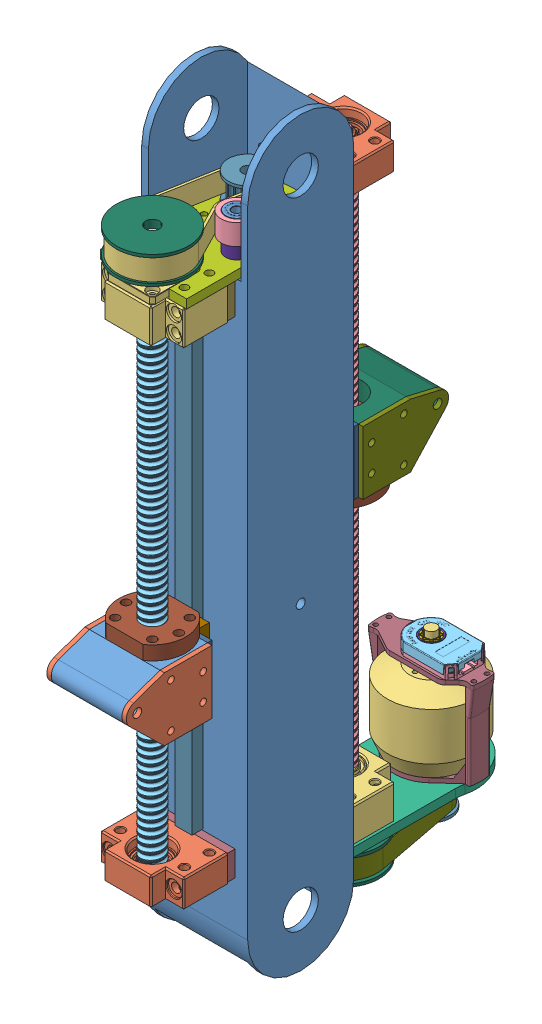
SolidWorks assembly Shoulder, configuration Default. Lengths in mm.
Overall size (98.94 610.39 280.38).
79 component instances, 40 part files, 66 mates.
Components (placement in the parent):
- Box^Shoulder-1: Box^Shoulder [Default] at origin size (76.2 533.4 76.2) (virtual)
- BF12-1: BF12 [Default] at (0 614.1315 -46.7041) x (1 0 0) z (0 1 0) size (60 43 20)
- BK12-1: BK12 [Default] at (0 212.1315 -46.7041) x (-1 0 0) z (0 -1 0) size (60 46.94 35.34)
- SFU1605-450-1: SFU1605-450 [1605-400] at (0 171.1315 -71.7041) x (1 0 0) z (0 -1 0) size (16.52 16.22 450)
- BK12-2: BK12 [Default] at (0 582.269 40.2909) x (-1 0 0) z (0 1 0) size (60 46.94 35.34)
- BF12-2: BF12 [Default] at (0 230.269 40.2909) x (-1 0 0) z (0 1 0) size (60 43 20)
- SFU1605-400-3: SFU1605-400 [1605-400] at (0 623.269 65.2909) x (-1 0 0) z (0 1 0) size (16.52 16.22 400)
- J3Plate^Shoulder-1: J3Plate^Shoulder [Default] at origin size (65 6.35 120.35) (virtual)
- J2Plate^Shoulder-1: J2Plate^Shoulder [Default] at origin size (66.67 6.35 116.57) (virtual)
- J3MGN12R-1: J3MGN12R [Default] at origin size (12 379.5 8)
- J3MGN12C-1: J3MGN12C [Default] at (0 433.1293 -49.3066) x (1 0 0) z (0 1 0) size (27 10 45.5)
- CarriagePlate^Shoulder-1: CarriagePlate^Shoulder [Default] at (0 67.1524 -3.2066) size (50.8 45.5 3.17) (virtual)
- nut-1: nut [Default] at (0 410.3793 -71.7041) x (-1 0 0) z (0 -1 0) size (48 40 42)
- BKSpacer^Shoulder-1: BKSpacer^Shoulder [Default] at origin size (58 23 5.4) (virtual)
- BKSpacer^Shoulder-2: BKSpacer^Shoulder [Default] at (0 370.1375 81.5975) size (58 23 5.4) (virtual)
- BFSpacer^Shoulder-1: BFSpacer^Shoulder [Default] at origin size (58 18 5.4) (virtual)
- BFSpacer^Shoulder-2: BFSpacer^Shoulder [Default] at (0 -383.8625 81.5975) size (58 18 5.4) (virtual)
- J2MGN12R^Shoulder-1: J2MGN12R^Shoulder [Default] at origin size (12 329.5 8) (virtual)
- J3Adapter^Shoulder-2: J3Adapter^Shoulder [Default] at (0 76.5186 -3.2066) size (57.15 45.79 61.61) (virtual)
  - Body^J3Adapter_Shoulder-1: Body^J3Adapter_Shoulder [Default] at (38.1 26.927 0) x (0 0 -1) z (1 0 0) size (61.61 45.5 50.8) (virtual)
  - SidePlate^J3Adapter_Shoulder-1: SidePlate^J3Adapter_Shoulder [Default] at origin size (3.18 45.5 61.61) (virtual)
  - SidePlate^J3Adapter_Shoulder-2: SidePlate^J3Adapter_Shoulder [Default] at (53.975 0 0) size (3.18 45.5 61.61) (virtual)
  - 94459A340_BRASS HEAT-SET INSERT FOR PLASTIC-1: 94459A340_BRASS HEAT-SET INSERT FOR PLASTIC [94459A340] at (-18.415 340.7357 -83.735) x (0 -1 0) z (0 0 -1) size (7.22 6.55 7.22)
  - 94459A220_BRASS HEAT-SET INSERT FOR PLASTIC-1: 94459A220_BRASS HEAT-SET INSERT FOR PLASTIC [94459A220] at (13.435 346.5607 -81.9325) x (-0.837169 0 -0.546944) z (-0.546944 0 0.837169) size (8.76 13.2 8.76)
- J3MGN12C-2: J3MGN12C [Default] at (0 351.2303 42.8934) x (-1 0 0) z (0 1 0) size (27 10 45.5)
- nut-2: nut [Default] at (0 373.9803 65.2909) x (1 0 0) z (0 1 0) size (48 40 42)
- J2Adapter^Shoulder-1: J2Adapter^Shoulder [Default] at (0 707.841 -3.2066) x (1 0 0) z (0 0 -1) size (57.15 457.2 153.99) (virtual)
  - Body^J2Adapter_Shoulder-1: Body^J2Adapter_Shoulder [Default] at (38.1 26.927 0) x (0 0 -1) z (1 0 0) size (61.61 45.5 50.8) (virtual)
  - SidePlate^J2Adapter_Shoulder-1: SidePlate^J2Adapter_Shoulder [Default] at origin size (3.18 45.5 61.61) (virtual)
  - SidePlate^J2Adapter_Shoulder-2: SidePlate^J2Adapter_Shoulder [Default] at (53.975 0 0) size (3.18 45.5 61.61) (virtual)
  - 94459A340_BRASS HEAT-SET INSERT FOR PLASTIC-1: 94459A340_BRASS HEAT-SET INSERT FOR PLASTIC [94459A340] at (-18.415 340.7357 -83.735) x (0 -1 0) z (0 0 -1) size (7.22 6.55 7.22)
  - 94459A220_BRASS HEAT-SET INSERT FOR PLASTIC-1: 94459A220_BRASS HEAT-SET INSERT FOR PLASTIC [94459A220] at (13.435 346.5607 -81.9325) x (-0.837169 0 -0.546944) z (-0.546944 0 0.837169) size (8.76 13.2 8.76)
- CarriagePlate^Shoulder-2: CarriagePlate^Shoulder [Default] at (0 -14.7465 -3.2066) x (-1 0 0) z (0 0 -1) size (50.8 45.5 3.17) (virtual)
- 192kvMotorEncoded-1: 192kvMotorEncoded [Default] at (0 202.8065 -135.2041) x (0 0 -1) z (1 0 0) size (63 104.52 76.93)
  - BetterKEDA-1: BetterKEDA [Default] at origin size (63 104.52 63)
  - CUI_DEVICES_AMT102-0048-N2000-S-1: CUI_DEVICES_AMT102-0048-N2000-S [Default] at (0 65.12 0) x (1 0 0) z (0 1 0) size (36.33 46.21 9.2)
    - CUI_DEVICES_AMT102-0048-N2000-S.step-1: CUI_DEVICES_AMT102-0048-N2000-S.step [Default] at origin size (36.33 46.21 9.2)
      - AMT-102-Base-REV-K.step-1: AMT-102-Base-REV-K.step [Default] x (-1 0 0) z (0 0 -1) size (28.78 43.39 9.06)
      - AMT-102-Top-Cover-REV-H.step-1: AMT-102-Top-Cover-REV-H.step [Default] at (0 0 5.23) x (-1 0 0) z (0 0 -1) size (28.6 43.26 6.55)
      - AMT-Sleeve-REV-D_ 2 mm.step-1: AMT-Sleeve-REV-D_ 2 mm.step [Default] at (0 0 -2.42) x (0.999996 0.002864 0) z (0 0 1) size (10.79 10.79 7.8)
      - AMT-Hub-Top-REV-D1.step-1: AMT-Hub-Top-REV-D1.step [Default] at (0 0 2.13) x (0.999996 0.002864 0) z (0 0 1) size (14 14 5.67)
      - AMT-Hub-Bottom-REV-B.step-1: AMT-Hub-Bottom-REV-B.step [Default] at (0 0 2.43) x (0.999998 -0.001942 0) z (0 0 1) size (17.3 17.3 3.2)
      - AMT10X-Shaft-Adaptor-REV-E.step-1: AMT10X-Shaft-Adaptor-REV-E.step [Default] at (0 0 0.03) x (0.999996 0.002864 0) z (0 0 1) size (11.8 11.8 7.8)
      - Receiver-board.step-1: Receiver-board.step [Default] at (72.2834 -20.351 3.03) x (-1 0 0) z (0 0 -1) size (26.5 26.62 0.41)
      - Rotor-board-REV F.step-1: Rotor-board-REV F.step [Default] at (0 0 2.13) x (0.807874 -0.589355 0) z (0 0 1) size (26 26 0.3)
      - Transmitter-board AMT10_AMT-102.step-1: Transmitter-board AMT10_AMT-102.step [Default] at (19.1596 -17.1102 1.22) x (-1 0 0) z (0 0 -1) size (26.63 38.43 4.41)
  - Body^192kvMotorEncoded-1: Body^192kvMotorEncoded [Default] at origin size (53 64.53 76.93) (virtual)
- 192kvMotorEncoded-2: 192kvMotorEncoded [Default] at (0 591.594 -3.2066) x (-0.707107 0 -0.707107) z (-0.707107 0 0.707107) size (63 104.52 76.93)
  - BetterKEDA-1: BetterKEDA [Default] at origin size (63 104.52 63)
  - CUI_DEVICES_AMT102-0048-N2000-S-1: CUI_DEVICES_AMT102-0048-N2000-S [Default] at (0 65.12 0) x (1 0 0) z (0 1 0) size (36.33 46.21 9.2)
    - CUI_DEVICES_AMT102-0048-N2000-S.step-1: CUI_DEVICES_AMT102-0048-N2000-S.step [Default] at origin size (36.33 46.21 9.2)
      - AMT-102-Base-REV-K.step-1: AMT-102-Base-REV-K.step [Default] x (-1 0 0) z (0 0 -1) size (28.78 43.39 9.06)
      - AMT-102-Top-Cover-REV-H.step-1: AMT-102-Top-Cover-REV-H.step [Default] at (0 0 5.23) x (-1 0 0) z (0 0 -1) size (28.6 43.26 6.55)
      - AMT-Sleeve-REV-D_ 2 mm.step-1: AMT-Sleeve-REV-D_ 2 mm.step [Default] at (0 0 -2.42) x (0.999996 0.002864 0) z (0 0 1) size (10.79 10.79 7.8)
      - AMT-Hub-Top-REV-D1.step-1: AMT-Hub-Top-REV-D1.step [Default] at (0 0 2.13) x (0.999996 0.002864 0) z (0 0 1) size (14 14 5.67)
      - AMT-Hub-Bottom-REV-B.step-1: AMT-Hub-Bottom-REV-B.step [Default] at (0 0 2.43) x (0.999998 -0.001942 0) z (0 0 1) size (17.3 17.3 3.2)
      - AMT10X-Shaft-Adaptor-REV-E.step-1: AMT10X-Shaft-Adaptor-REV-E.step [Default] at (0 0 0.03) x (0.999996 0.002864 0) z (0 0 1) size (11.8 11.8 7.8)
      - Receiver-board.step-1: Receiver-board.step [Default] at (72.2834 -20.351 3.03) x (-1 0 0) z (0 0 -1) size (26.5 26.62 0.41)
      - Rotor-board-REV F.step-1: Rotor-board-REV F.step [Default] at (0 0 2.13) x (0.807874 -0.589355 0) z (0 0 1) size (26 26 0.3)
      - Transmitter-board AMT10_AMT-102.step-1: Transmitter-board AMT10_AMT-102.step [Default] at (19.1596 -17.1102 1.22) x (-1 0 0) z (0 0 -1) size (26.63 38.43 4.41)
  - Body^192kvMotorEncoded-1: Body^192kvMotorEncoded [Default] at origin size (53 64.53 76.93) (virtual)
- 15Tpulley-3: 15Tpulley [Default] at (0 175.8815 -135.2041) size (28 28 28)
- 15Tpulley-4: 15Tpulley [Default] at (0 618.519 -3.2066) x (-1 0 0) z (0 0 1) size (28 28 28)
- 30Tpulley-3: 30Tpulley [Default] at (0 618.519 65.2909) size (52 20 52)
- 30Tpulley-4: 30Tpulley [Default] at (0 175.8815 -71.7041) size (52 20 52)
- J3Belt^Shoulder-1: J3Belt^Shoulder [Default] at origin size (49.49 15 101.05) (virtual)
- TensionPillarJ3-1: TensionPillarJ3 [Default] at (-42.5291 257.8915 3.8215) size (22.22 25.73 22.23)
  - 92510A774_ALUM UNTHRD SPACER-1-1: 92510A774_ALUM UNTHRD SPACER-1 [92510A774] at (20.3041 -69.3725 -110.4505) x (1 0 0) z (0 1 0) size (15.88 15.88 9.53)
  - 98019A228_MIL SPEC. 300 SERIES SS FLAT WASHER-1: 98019A228_MIL SPEC. 300 SERIES SS FLAT WASHER [98019A228] at (20.3041 -74.8462 -110.4505) x (0.972939 0 -0.231063) z (0.231063 0 0.972939) size (9.53 0.71 9.53)
  - 60355K701_BALL BEARING-1: 60355K701_BALL BEARING [60355K701] at (20.3041 -77.3354 -110.4505) x (1 0 0) z (0 1 0) size (15.88 15.88 4.98)
  - Roller^TensionPillarJ3-1: Roller^TensionPillarJ3 [Default] at (-2.0675 -17.1652 2.6827) size (22.23 15 22.23) (virtual)
  - 60355K701_BALL BEARING-2: 60355K701_BALL BEARING [60355K701] at (20.3041 -87.8548 -110.4505) x (1 0 0) z (0 1 0) size (15.88 15.88 4.98)
- J2Belt^Shoulder-1: J2Belt^Shoulder [Default] at origin size (49.49 15 106.05) (virtual)
- TensionPillarJ2-1: TensionPillarJ2 [Default] at (-24.3623 536.509 127.3519) x (-0.837169 0 -0.546944) z (-0.546944 0 0.837169) size (22.22 25.73 22.23)
  - 92510A774_ALUM UNTHRD SPACER-1-1: 92510A774_ALUM UNTHRD SPACER-1 [92510A774] at (20.3041 -69.3725 -110.4505) x (1 0 0) z (0 1 0) size (15.88 15.88 9.53)
  - 98019A228_MIL SPEC. 300 SERIES SS FLAT WASHER-1: 98019A228_MIL SPEC. 300 SERIES SS FLAT WASHER [98019A228] at (20.3041 -74.8462 -110.4505) x (0.972939 0 -0.231063) z (0.231063 0 0.972939) size (9.53 0.71 9.53)
  - 60355K701_BALL BEARING-1: 60355K701_BALL BEARING [60355K701] at (20.3041 -77.3354 -110.4505) x (1 0 0) z (0 1 0) size (15.88 15.88 4.98)
  - Roller^TensionPillarJ2-1: Roller^TensionPillarJ2 [Default] at (-2.0675 -17.1652 2.6827) size (22.23 15 22.23) (virtual)
  - 60355K701_BALL BEARING-2: 60355K701_BALL BEARING [60355K701] at (20.3041 -87.8548 -110.4505) x (1 0 0) z (0 1 0) size (15.88 15.88 4.98)
Mates (geometry in assembly coordinates):
- Parallel1: parallel anti-aligned: plane of Box^Shoulder-1 through (-33.3375 186.9315 -41.3066) normal (0 0 -1); plane of BF12-1 through (29 605.1315 -46.7041) normal (0 0 1)
- Width1: width anti-aligned: plane of BF12-1 through (30 605.1315 -78.2041) normal (1 0 0); plane of Box^Shoulder-1 through (-30 605.1315 -47.7041) normal (-1 0 0); plane of BF12-1 through (38.1 644.1315 -3.2066) normal (1 0 0); plane of Box^Shoulder-1 through (-38.1 186.9315 -3.2066) normal (-1 0 0)
- Distance6: distance anti-aligned: plane of Box^Shoulder-1 through (-33.3375 186.9315 -41.3066) normal (0 0 -1); plane of BK12-1 through (-29 223.6315 -46.7041) normal (0 0 1)
- Width2: width aligned: plane of BK12-1 through (30 223.6315 -47.7041) normal (1 0 0); plane of Box^Shoulder-1 through (-30 223.6315 -78.2041) normal (-1 0 0); plane of BK12-1 through (-38.1 186.9315 -3.2066) normal (-1 0 0); plane of Box^Shoulder-1 through (38.1 644.1315 -3.2066) normal (1 0 0)
- Parallel3: parallel aligned: plane of BK12-1 through (29 224.6315 -47.7041) normal (0 1 0)
- Coincident11: coincident: line of SFU1605-450-1 through (0 185.8815 -71.7041) axis (0 -1 0)
- Concentric6: concentric anti-aligned: cylinder of BK12-1 through (0 220.1315 -71.7041) axis (0 1 0) radius 6; cylinder of SFU1605-450-1 through (0 186.1315 -71.7041) axis (0 -1 0) radius 5
- Coincident12: coincident anti-aligned: plane of BK12-1 through (7.2358 225.1315 -64.4683) normal (0 1 0); plane of SFU1605-450-1 through (0 225.1315 -71.7041) normal (0 -1 0)
- Coincident13: coincident anti-aligned: plane of BF12-1 through (-6.5021 610.1315 -65.202) normal (0 -1 0); plane of SFU1605-450-1 through (0 610.1315 -71.7041) normal (0 1 0)
- Distance3: distance = 12.7 mm: plane of BK12-1 through (29 199.6315 -47.7041) normal (0 -1 0); line of Box^Shoulder-1 through (38.1 186.9315 -41.3066) axis (-1 0 0)
- Coincident27: coincident: line of SFU1605-400-3 through (0 608.519 65.2909) axis (0 1 0)
- Concentric18: concentric anti-aligned: cylinder of BK12-2 through (0 582.269 65.2909) axis (0 -1 0) radius 6; cylinder of SFU1605-400-3 through (0 608.269 65.2909) axis (0 1 0) radius 5
- Distance8: distance anti-aligned: plane of Box^Shoulder-1 through (-33.3375 186.9315 34.8934) normal (0 0 1); plane of BK12-2 through (-29 570.769 40.2909) normal (0 0 -1)
- Coincident29: coincident anti-aligned: plane of BK12-2 through (7.2358 569.269 58.0551) normal (0 -1 0); plane of SFU1605-400-3 through (0 569.269 65.2909) normal (0 1 0)
- Coincident30: coincident anti-aligned: plane of BF12-2 through (-6.5021 234.269 58.7888) normal (0 1 0); plane of SFU1605-400-3 through (0 234.269 65.2909) normal (0 -1 0)
- Concentric19: concentric anti-aligned: cylinder of BF12-2 through (0 227.069 65.2909) axis (0 1 0) radius 5; cylinder of SFU1605-400-3 through (0 234.269 65.2909) axis (0 -1 0) radius 5
- Distance5: distance = 33.3375 mm: line of Box^Shoulder-1 through (38.1 186.9315 34.8934) axis (-1 0 0); plane of BF12-2 through (29 220.269 41.2909) normal (0 -1 0)
- Coincident35: coincident anti-aligned: plane of J3MGN12R-1 through (0 0 -49.3066) normal (0 0 -1); plane of J3MGN12C-1 through (-6 455.8793 -49.3066) normal (0 0 1)
- Width3: width anti-aligned: plane of J3MGN12C-1 through (13.5 455.8793 -44.3066) normal (1 0 0); plane of J3MGN12C-1 through (-13.5 455.8793 -44.3066) normal (-1 0 0); plane of J3MGN12R-1 through (-6 604.1315 -49.3066) normal (-1 0 0); plane of J3MGN12R-1 through (6 604.1315 -49.3066) normal (1 0 0)
- Coincident36: coincident anti-aligned: plane of J3MGN12C-1 through (13.5 455.8793 -54.3066) normal (0 0 -1); plane of CarriagePlate^Shoulder-1 through (0 67.1524 -54.3066) normal (0 0 1)
- Concentric22: concentric anti-aligned: cylinder of J3MGN12C-1 through (10 443.1293 -50.3066) axis (0 0 -1) radius 1.5; cylinder of CarriagePlate^Shoulder-1 through (10 443.1293 -57.4816) axis (0 0 1) radius 1.5
- Concentric23: concentric anti-aligned: cylinder of J3MGN12C-1 through (-10 423.1293 -50.3066) axis (0 0 -1) radius 1.5; cylinder of CarriagePlate^Shoulder-1 through (-10 423.1293 -57.4816) axis (0 0 1) radius 1.5
- Concentric24: concentric aligned: cylinder of SFU1605-450-1 through (0 610.1315 -71.7041) axis (0 1 0) radius 5; cylinder of nut-1 through (0 400.3793 -71.7041) axis (0 1 0) radius 8
- Concentric25: concentric aligned: cylinder of BF12-1 through (0 610.9315 -71.7041) axis (0 1 0) radius 5; cylinder of SFU1605-450-1 through (0 610.1315 -71.7041) axis (0 1 0) radius 5
- Coincident37: coincident anti-aligned: plane of CarriagePlate^Shoulder-1 through (-25.4 410.3793 -57.4816) normal (0 -1 0); plane of nut-1 through (0 410.3793 -71.7041) normal (0 1 0)
- Parallel4: parallel anti-aligned: plane of Box^Shoulder-1 through (-33.3375 186.9315 34.8934) normal (0 0 1); plane of BF12-2 through (-29 221.269 40.2909) normal (0 0 -1)
- Concentric27: concentric anti-aligned: cylinder of BK12-2 through (-23 575.769 40.2909) axis (0 0 1) radius 3.3; cylinder of BKSpacer^Shoulder-2 through (-23 575.769 102.6848) axis (0 0 -1) radius 3.3
- Concentric28: concentric anti-aligned: cylinder of BK12-2 through (23 575.769 40.2909) axis (0 0 1) radius 3.3; cylinder of BKSpacer^Shoulder-2 through (23 575.769 102.6848) axis (0 0 -1) radius 3.3
- Coincident42: coincident anti-aligned: plane of Box^Shoulder-1 through (-33.3375 186.9315 34.8934) normal (0 0 1); plane of BKSpacer^Shoulder-2 through (0 370.1375 34.8934) normal (0 0 -1)
- Concentric29: concentric anti-aligned: cylinder of BF12-2 through (23 230.269 40.2909) axis (0 0 1) radius 3.3; cylinder of BFSpacer^Shoulder-2 through (23 230.269 101.0198) axis (0 0 -1) radius 3.3
- Concentric30: concentric anti-aligned: cylinder of BF12-2 through (-23 230.269 40.2909) axis (0 0 1) radius 3.3; cylinder of BFSpacer^Shoulder-2 through (-23 230.269 101.0198) axis (0 0 -1) radius 3.3
- Coincident43: coincident anti-aligned: plane of Box^Shoulder-1 through (-33.3375 186.9315 34.8934) normal (0 0 1); plane of BFSpacer^Shoulder-2 through (0 -383.8625 34.8934) normal (0 0 -1)
- Concentric32: concentric anti-aligned: cylinder of nut-1 through (0 442.3793 -71.7041) axis (0 -1 0) radius 14; cylinder of Adapter^Shoulder-2/Body^Adapter_Shoulder-1 through (0 349.1272 -71.7041) axis (0 1 0) radius 14
- Parallel6: parallel anti-aligned: plane of CarriagePlate^Shoulder-1 through (0 67.1524 -57.4816) normal (0 0 -1); plane of Adapter^Shoulder-2/Body^Adapter_Shoulder-1 through (38.1 349.1272 -57.4816) normal (0 0 1)
- Coincident47: coincident anti-aligned: plane of nut-1 through (0 410.3793 -71.7041) normal (0 1 0); plane of Adapter^Shoulder-2/Body^Adapter_Shoulder-1 through (-25.4 410.3793 -57.4816) normal (0 -1 0)
- Coincident48: coincident anti-aligned: plane of nut-1 through (0 410.3793 -71.7041) normal (0 1 0); plane of Adapter^Shoulder-2/Body^Adapter_Shoulder-1 through (-25.4 410.3793 -57.4816) normal (0 -1 0)
- Coincident49: coincident anti-aligned: plane of nut-1 through (0 410.3793 -71.7041) normal (0 1 0); plane of Adapter^Shoulder-2/Body^Adapter_Shoulder-1 through (-25.4 410.3793 -57.4816) normal (0 -1 0)
- Coincident51: coincident anti-aligned: plane of J2MGN12R^Shoulder-1 through (0 0 42.8934) normal (0 0 1); plane of J3MGN12C-2 through (6 373.9803 42.8934) normal (0 0 -1)
- Width6: width anti-aligned: plane of J3MGN12C-2 through (-13.5 373.9803 37.8934) normal (-1 0 0); plane of J3MGN12C-2 through (13.5 373.9803 37.8934) normal (1 0 0); plane of J2MGN12R^Shoulder-1 through (6 569.769 42.8934) normal (1 0 0); plane of J2MGN12R^Shoulder-1 through (-6 569.769 42.8934) normal (-1 0 0)
- Concentric34: concentric anti-aligned: cylinder of SFU1605-400-3 through (0 608.269 65.2909) axis (0 1 0) radius 5; cylinder of nut-2 through (0 383.9803 65.2909) axis (0 -1 0) radius 8
- Coincident52: coincident anti-aligned: plane of J3MGN12C-2 through (0 373.9803 42.8934) normal (0 1 0); plane of nut-2 through (0 373.9803 65.2909) normal (0 -1 0)
- Concentric35: concentric anti-aligned: cylinder of nut-2 through (0 341.9803 65.2909) axis (0 1 0) radius 14; cylinder of J2Adapter^Shoulder-1/Body^J2Adapter_Shoulder-1 through (0 435.2324 65.2909) axis (0 -1 0) radius 14
- Parallel7: parallel anti-aligned: plane of J3MGN12C-2 through (-13.5 373.9803 47.8934) normal (0 0 1); plane of J2Adapter^Shoulder-1/Body^J2Adapter_Shoulder-1 through (38.1 435.2324 51.0684) normal (0 0 -1)
- Coincident54: coincident anti-aligned: plane of nut-2 through (0 373.9803 65.2909) normal (0 -1 0); plane of J2Adapter^Shoulder-1/Body^J2Adapter_Shoulder-1 through (-25.4 373.9803 51.0684) normal (0 1 0)
- Concentric36: concentric anti-aligned: cylinder of J3MGN12C-2 through (10 361.2303 43.8934) axis (0 0 1) radius 1.5; cylinder of CarriagePlate^Shoulder-2 through (10 361.2303 51.0684) axis (0 0 -1) radius 1.5
- Concentric37: concentric anti-aligned: cylinder of J3MGN12C-2 through (-10 341.2303 43.8934) axis (0 0 1) radius 1.5; cylinder of CarriagePlate^Shoulder-2 through (-10 341.2303 51.0684) axis (0 0 -1) radius 1.5
- Coincident55: coincident anti-aligned: plane of J3MGN12C-2 through (-13.5 373.9803 47.8934) normal (0 0 1); plane of CarriagePlate^Shoulder-2 through (0 -14.7465 47.8934) normal (0 0 -1)
- Parallel8: parallel aligned: plane of BF12-2 through (29 240.269 41.2909) normal (0 1 0)
- Concentric38: concentric aligned: cylinder of J3Plate^Shoulder-1 through (0 193.2815 -135.2041) axis (0 1 0) radius 15.875; cylinder of 192kvMotorEncoded-1/BetterKEDA-1 through (0 173.2815 -135.2041) axis (0 1 0) radius 4
- Concentric39: concentric aligned: cylinder of J3Plate^Shoulder-1 through (0 193.2815 -113.0041) axis (0 1 0) radius 2; cylinder of 192kvMotorEncoded-1/Body^192kvMotorEncoded-1 through (0 199.6315 -113.0041) axis (0 1 0) radius 2
- Coincident56: coincident anti-aligned: plane of J3Plate^Shoulder-1 through (56.3375 199.6315 -121.8438) normal (0 1 0); plane of 192kvMotorEncoded-1/Body^192kvMotorEncoded-1 through (0 199.6315 -135.2041) normal (0 -1 0)
- Concentric40: concentric aligned: cylinder of J2Plate^Shoulder-1 through (0 601.119 -3.2066) axis (0 -1 0) radius 15.875; cylinder of 192kvMotorEncoded-2/BetterKEDA-1 through (0 621.119 -3.2066) axis (0 -1 0) radius 4
- Concentric41: concentric aligned: cylinder of J2Plate^Shoulder-1 through (-15.6978 601.119 12.4912) axis (0 -1 0) radius 2; cylinder of 192kvMotorEncoded-2/Body^192kvMotorEncoded-1 through (-15.6978 594.769 12.4912) axis (0 -1 0) radius 2
- Coincident57: coincident anti-aligned: plane of J2Plate^Shoulder-1 through (0 594.769 0) normal (0 -1 0); plane of 192kvMotorEncoded-2/Body^192kvMotorEncoded-1 through (0 594.769 -3.2066) normal (0 1 0)
- Concentric42: concentric anti-aligned: cylinder of 192kvMotorEncoded-1/BetterKEDA-1 through (0 173.2815 -135.2041) axis (0 1 0) radius 4; cylinder of 15Tpulley-3 through (0 183.8815 -135.2041) axis (0 -1 0) radius 4
- Concentric44: concentric anti-aligned: cylinder of 192kvMotorEncoded-2/BetterKEDA-1 through (0 621.119 -3.2066) axis (0 -1 0) radius 4; cylinder of 15Tpulley-4 through (0 610.519 -3.2066) axis (0 1 0) radius 4
- Concentric45: concentric anti-aligned: cylinder of SFU1605-400-3 through (0 608.269 65.2909) axis (0 1 0) radius 5; cylinder of 30Tpulley-3 through (0 626.519 65.2909) axis (0 -1 0) radius 5
- Coincident61: coincident anti-aligned: circle of SFU1605-400-3; plane of 30Tpulley-3 through (0 608.519 65.2909) normal (0 -1 0)
- Coincident62: coincident aligned: plane of 15Tpulley-4 through (0 626.519 -3.2066) normal (0 -1 0); plane of 30Tpulley-3 through (0 626.519 65.2909) normal (0 -1 0)
- Concentric47: concentric aligned: cylinder of SFU1605-450-1 through (0 186.1315 -71.7041) axis (0 -1 0) radius 5; cylinder of 30Tpulley-4 through (0 183.8815 -71.7041) axis (0 -1 0) radius 5
- Coincident63: coincident anti-aligned: circle of SFU1605-450-1; plane of 30Tpulley-4 through (0 185.8815 -71.7041) normal (0 1 0)
- Coincident64: coincident aligned: plane of 15Tpulley-3 through (0 167.8815 -135.2041) normal (0 1 0); plane of 30Tpulley-4 through (0 167.8815 -71.7041) normal (0 1 0)
- Concentric48: concentric aligned: cylinder of J3Plate^Shoulder-1 through (-22.225 199.6315 -106.6291) axis (0 -1 0) radius 3.175; cylinder of TensionPillarJ3-1/92510A774_ALUM UNTHRD SPACER-1-1 through (-22.225 193.2815 -106.6291) axis (0 -1 0) radius 3.2004
- Coincident65: coincident anti-aligned: plane of J3Plate^Shoulder-1 through (56.3375 193.2815 -121.8438) normal (0 -1 0); plane of TensionPillarJ3-1/92510A774_ALUM UNTHRD SPACER-1-1 through (-22.225 193.2815 -106.6291) normal (0 1 0)
- Concentric49: concentric aligned: cylinder of J2Plate^Shoulder-1 through (19.05 587.4052 23.7809) axis (0 1 0) radius 2.6035; cylinder of TensionPillarJ2-1/92510A774_ALUM UNTHRD SPACER-1-1 through (19.05 601.119 23.7809) axis (0 1 0) radius 3.2004
- Coincident66: coincident anti-aligned: plane of J2Plate^Shoulder-1 through (0 601.119 0) normal (0 1 0); plane of TensionPillarJ2-1/92510A774_ALUM UNTHRD SPACER-1-1 through (19.05 601.119 23.7809) normal (0 -1 0)
